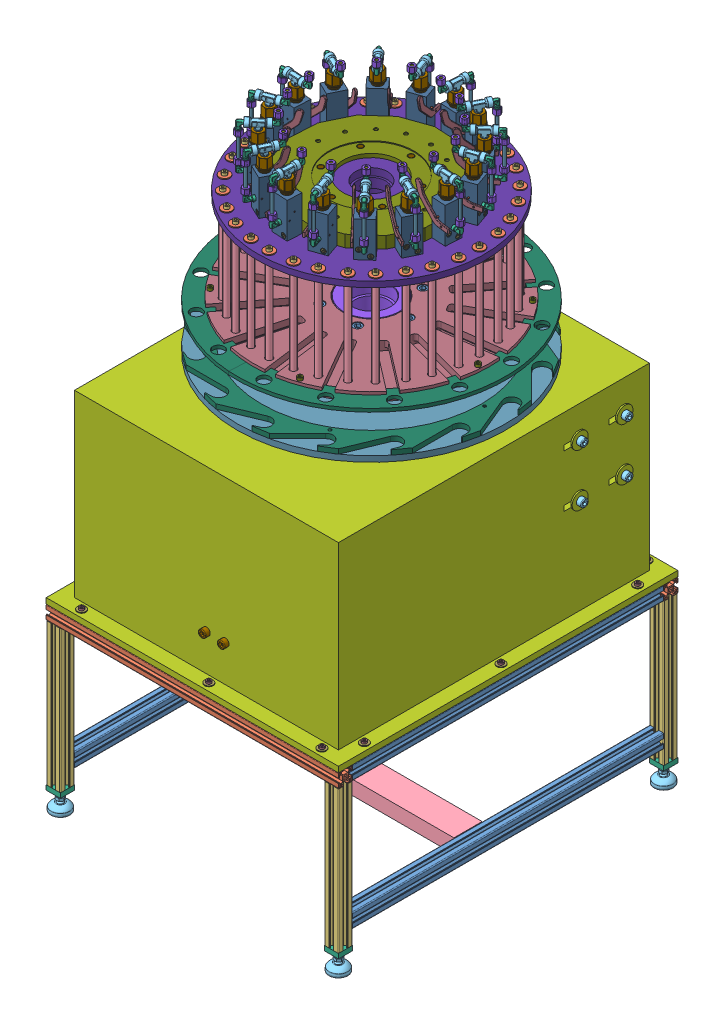
SolidWorks assembly Assieme_FINALE, configuration Default. Lengths in mm. (continued)
Components (placement in the parent): (continued)
- assieme parte rotante-1: assieme parte rotante [Default] at (-376.3498 623.9178 -790.5811) x (0 1 0) z (0 0 1) size (749.63 778.63 778.63) (continued)
  - AssiemeValvola-4: AssiemeValvola [Default] at (515.3257 -108.3081 301.6234) x (0 0.745128 0.666921) z (0 0.666921 -0.745128) size (90.26 138.63 38) (continued)
    - Raccordo a L-3: Raccordo a L [Default] at (-30 -88.2824 0) x (0 1 0) z (0 0 1) size (28.34 25.51 14.01)
      - 1809_06_10_01-1: 1809_06_10_01 [Default] at origin size (22.49 23 10)
      - 1809_06_10_02-1: 1809_06_10_02 [Default] at origin size (6.5 8.5 8.5)
      - 1809_06_10_03-1: 1809_06_10_03 [Default] at origin size (11.02 15.01 14.01)
    - Spina_3x38-1: Spina_3x38 [Default] at (0 -68.2824 -21) x (-1 0 0) z (0 0 1) size (3 3 38)
    - Spina_3x38-2: Spina_3x38 [Default] at (-10 -80.2824 -21) x (0.996193 0.087174 0) z (0 0 1) size (3 3 38)
    - M5 40mm-3: M5 40mm [ISO 4762 M5 x 40 - 40N] at (-14.6 -108.7824 9) size (45 8.5 8.5)
    - M5 40mm-2: M5 40mm [ISO 4762 M5 x 40 - 40N] at (-14.6 -96.7824 -9) size (45 8.5 8.5)
    - LevaValvola-1: LevaValvola [Default] at (-24.507 -86.571 -17) x (0.996193 0.087174 0) z (0 0 1) size (77.55 60.2 4)
    - Tubo-1: Tubo [Default] at (-30 -15.9665 0) x (1 0 0) z (0 -1 0) size (6 6 56.4)
  - AssiemeValvola-5: AssiemeValvola [Default] at (515.3257 -142.0531 358.7289) x (0 0.943628 0.331007) z (0 0.331007 -0.943628) size (90.26 138.63 38)
    - RaccordoT-1: RaccordoT [Default] at origin size (43 29.75 16.5)
    - Raccordo a L-1: Raccordo a L [Default] at (-30 0 0) x (0 -1 0) z (0 0 -1) size (28.34 25.51 14.01)
      - 1809_06_10_01-1: 1809_06_10_01 [Default] at origin size (22.49 23 10)
      - 1809_06_10_02-1: 1809_06_10_02 [Default] at origin size (6.5 8.5 8.5)
      - 1809_06_10_03-1: 1809_06_10_03 [Default] at origin size (11.02 15.01 14.01)
    - Raccordo a L-2: Raccordo a L [Default] at (30 0 0) x (0 1 0) z (0 0 -1) size (28.34 25.51 14.01)
      - 1809_06_10_01-1: 1809_06_10_01 [Default] at origin size (22.49 23 10)
      - 1809_06_10_02-1: 1809_06_10_02 [Default] at origin size (6.5 8.5 8.5)
      - 1809_06_10_03-1: 1809_06_10_03 [Default] at origin size (11.02 15.01 14.01)
    - TappoChiusura-1: TappoChiusura [Default] at (0 -32 0) x (0 -1 0) z (0 0 1) size (38.28 26.74 26.74)
    - CorpoValvola-1: CorpoValvola [Default] at (-15 -115.2824 0) size (30 75 34)
    - Raccordo a L-3: Raccordo a L [Default] at (-30 -88.2824 0) x (0 1 0) z (0 0 1) size (28.34 25.51 14.01)
      - 1809_06_10_01-1: 1809_06_10_01 [Default] at origin size (22.49 23 10)
      - 1809_06_10_02-1: 1809_06_10_02 [Default] at origin size (6.5 8.5 8.5)
      - 1809_06_10_03-1: 1809_06_10_03 [Default] at origin size (11.02 15.01 14.01)
    - Spina_3x38-1: Spina_3x38 [Default] at (0 -68.2824 -21) x (-1 0 0) z (0 0 1) size (3 3 38)
    - Spina_3x38-2: Spina_3x38 [Default] at (-10 -80.2824 -21) x (0.996193 0.087174 0) z (0 0 1) size (3 3 38)
    - M5 40mm-3: M5 40mm [ISO 4762 M5 x 40 - 40N] at (-14.6 -108.7824 9) size (45 8.5 8.5)
    - M5 40mm-2: M5 40mm [ISO 4762 M5 x 40 - 40N] at (-14.6 -96.7824 -9) size (45 8.5 8.5)
    - LevaValvola-1: LevaValvola [Default] at (-24.507 -86.571 -17) x (0.996193 0.087174 0) z (0 0 1) size (77.55 60.2 4)
    - Tubo-1: Tubo [Default] at (-30 -15.9665 0) x (1 0 0) z (0 -1 0) size (6 6 56.4)
  - AssiemeValvola-6: AssiemeValvola [Default] at (515.3257 -151.3762 424.4011) x (0 0.99847 -0.055301) z (0 -0.055301 -0.99847) size (90.26 138.63 38)
    - RaccordoT-1: RaccordoT [Default] at origin size (43 29.75 16.5)
    - Raccordo a L-1: Raccordo a L [Default] at (-30 0 0) x (0 -1 0) z (0 0 -1) size (28.34 25.51 14.01)
      - 1809_06_10_01-1: 1809_06_10_01 [Default] at origin size (22.49 23 10)
      - 1809_06_10_02-1: 1809_06_10_02 [Default] at origin size (6.5 8.5 8.5)
      - 1809_06_10_03-1: 1809_06_10_03 [Default] at origin size (11.02 15.01 14.01)
    - Raccordo a L-2: Raccordo a L [Default] at (30 0 0) x (0 1 0) z (0 0 -1) size (28.34 25.51 14.01)
      - 1809_06_10_01-1: 1809_06_10_01 [Default] at origin size (22.49 23 10)
      - 1809_06_10_02-1: 1809_06_10_02 [Default] at origin size (6.5 8.5 8.5)
      - 1809_06_10_03-1: 1809_06_10_03 [Default] at origin size (11.02 15.01 14.01)
    - TappoChiusura-1: TappoChiusura [Default] at (0 -32 0) x (0 -1 0) z (0 0 1) size (38.28 26.74 26.74)
    - CorpoValvola-1: CorpoValvola [Default] at (-15 -115.2824 0) size (30 75 34)
    - Raccordo a L-3: Raccordo a L [Default] at (-30 -88.2824 0) x (0 1 0) z (0 0 1) size (28.34 25.51 14.01)
      - 1809_06_10_01-1: 1809_06_10_01 [Default] at origin size (22.49 23 10)
      - 1809_06_10_02-1: 1809_06_10_02 [Default] at origin size (6.5 8.5 8.5)
      - 1809_06_10_03-1: 1809_06_10_03 [Default] at origin size (11.02 15.01 14.01)
    - Spina_3x38-1: Spina_3x38 [Default] at (0 -68.2824 -21) x (-1 0 0) z (0 0 1) size (3 3 38)
    - Spina_3x38-2: Spina_3x38 [Default] at (-10 -80.2824 -21) x (0.996193 0.087174 0) z (0 0 1) size (3 3 38)
    - M5 40mm-3: M5 40mm [ISO 4762 M5 x 40 - 40N] at (-14.6 -108.7824 9) size (45 8.5 8.5)
    - M5 40mm-2: M5 40mm [ISO 4762 M5 x 40 - 40N] at (-14.6 -96.7824 -9) size (45 8.5 8.5)
    - LevaValvola-1: LevaValvola [Default] at (-24.507 -86.571 -17) x (0.996193 0.087174 0) z (0 0 1) size (77.55 60.2 4)
    - Tubo-1: Tubo [Default] at (-30 -15.9665 0) x (1 0 0) z (0 -1 0) size (6 6 56.4)
  - AssiemeValvola-7: AssiemeValvola [Default] at (515.3257 -134.8578 488.6421) x (0 0.901303 -0.433189) z (0 -0.433189 -0.901303) size (90.26 138.63 38)
    - RaccordoT-1: RaccordoT [Default] at origin size (43 29.75 16.5)
    - Raccordo a L-1: Raccordo a L [Default] at (-30 0 0) x (0 -1 0) z (0 0 -1) size (28.34 25.51 14.01)
      - 1809_06_10_01-1: 1809_06_10_01 [Default] at origin size (22.49 23 10)
      - 1809_06_10_02-1: 1809_06_10_02 [Default] at origin size (6.5 8.5 8.5)
      - 1809_06_10_03-1: 1809_06_10_03 [Default] at origin size (11.02 15.01 14.01)
    - Raccordo a L-2: Raccordo a L [Default] at (30 0 0) x (0 1 0) z (0 0 -1) size (28.34 25.51 14.01)
      - 1809_06_10_01-1: 1809_06_10_01 [Default] at origin size (22.49 23 10)
      - 1809_06_10_02-1: 1809_06_10_02 [Default] at origin size (6.5 8.5 8.5)
      - 1809_06_10_03-1: 1809_06_10_03 [Default] at origin size (11.02 15.01 14.01)
    - TappoChiusura-1: TappoChiusura [Default] at (0 -32 0) x (0 -1 0) z (0 0 1) size (38.28 26.74 26.74)
    - CorpoValvola-1: CorpoValvola [Default] at (-15 -115.2824 0) size (30 75 34)
    - Raccordo a L-3: Raccordo a L [Default] at (-30 -88.2824 0) x (0 1 0) z (0 0 1) size (28.34 25.51 14.01)
      - 1809_06_10_01-1: 1809_06_10_01 [Default] at origin size (22.49 23 10)
      - 1809_06_10_02-1: 1809_06_10_02 [Default] at origin size (6.5 8.5 8.5)
      - 1809_06_10_03-1: 1809_06_10_03 [Default] at origin size (11.02 15.01 14.01)
    - Spina_3x38-1: Spina_3x38 [Default] at (0 -68.2824 -21) x (-1 0 0) z (0 0 1) size (3 3 38)
    - Spina_3x38-2: Spina_3x38 [Default] at (-10 -80.2824 -21) x (0.996193 0.087174 0) z (0 0 1) size (3 3 38)
    - M5 40mm-3: M5 40mm [ISO 4762 M5 x 40 - 40N] at (-14.6 -108.7824 9) size (45 8.5 8.5)
    - M5 40mm-2: M5 40mm [ISO 4762 M5 x 40 - 40N] at (-14.6 -96.7824 -9) size (45 8.5 8.5)
    - LevaValvola-1: LevaValvola [Default] at (-24.507 -86.571 -17) x (0.996193 0.087174 0) z (0 0 1) size (77.55 60.2 4)
    - Tubo-1: Tubo [Default] at (-30 -15.9665 0) x (1 0 0) z (0 -1 0) size (6 6 56.4)
  - AssiemeValvola-8: AssiemeValvola [Default] at (515.3257 -95.0129 541.6718) x (0 0.666921 -0.745128) z (0 -0.745128 -0.666921) size (90.26 138.63 38)
    - RaccordoT-1: RaccordoT [Default] at origin size (43 29.75 16.5)
    - Raccordo a L-1: Raccordo a L [Default] at (-30 0 0) x (0 -1 0) z (0 0 -1) size (28.34 25.51 14.01)
      - 1809_06_10_01-1: 1809_06_10_01 [Default] at origin size (22.49 23 10)
      - 1809_06_10_02-1: 1809_06_10_02 [Default] at origin size (6.5 8.5 8.5)
      - 1809_06_10_03-1: 1809_06_10_03 [Default] at origin size (11.02 15.01 14.01)
    - Raccordo a L-2: Raccordo a L [Default] at (30 0 0) x (0 1 0) z (0 0 -1) size (28.34 25.51 14.01)
      - 1809_06_10_01-1: 1809_06_10_01 [Default] at origin size (22.49 23 10)
      - 1809_06_10_02-1: 1809_06_10_02 [Default] at origin size (6.5 8.5 8.5)
      - 1809_06_10_03-1: 1809_06_10_03 [Default] at origin size (11.02 15.01 14.01)
    - TappoChiusura-1: TappoChiusura [Default] at (0 -32 0) x (0 -1 0) z (0 0 1) size (38.28 26.74 26.74)
    - CorpoValvola-1: CorpoValvola [Default] at (-15 -115.2824 0) size (30 75 34)
    - Raccordo a L-3: Raccordo a L [Default] at (-30 -88.2824 0) x (0 1 0) z (0 0 1) size (28.34 25.51 14.01)
      - 1809_06_10_01-1: 1809_06_10_01 [Default] at origin size (22.49 23 10)
      - 1809_06_10_02-1: 1809_06_10_02 [Default] at origin size (6.5 8.5 8.5)
      - 1809_06_10_03-1: 1809_06_10_03 [Default] at origin size (11.02 15.01 14.01)
    - Spina_3x38-1: Spina_3x38 [Default] at (0 -68.2824 -21) x (-1 0 0) z (0 0 1) size (3 3 38)
    - Spina_3x38-2: Spina_3x38 [Default] at (-10 -80.2824 -21) x (0.996193 0.087174 0) z (0 0 1) size (3 3 38)
    - M5 40mm-3: M5 40mm [ISO 4762 M5 x 40 - 40N] at (-14.6 -108.7824 9) size (45 8.5 8.5)
    - M5 40mm-2: M5 40mm [ISO 4762 M5 x 40 - 40N] at (-14.6 -96.7824 -9) size (45 8.5 8.5)
    - LevaValvola-1: LevaValvola [Default] at (-24.507 -86.571 -17) x (0.996193 0.087174 0) z (0 0 1) size (77.55 60.2 4)
    - Tubo-1: Tubo [Default] at (-30 -15.9665 0) x (1 0 0) z (0 -1 0) size (6 6 56.4)
  - AssiemeValvola-9: AssiemeValvola [Default] at (515.3257 -37.9074 575.4168) x (0 0.331007 -0.943628) z (0 -0.943628 -0.331007) size (90.26 138.63 38)
    - RaccordoT-1: RaccordoT [Default] at origin size (43 29.75 16.5)
    - Raccordo a L-1: Raccordo a L [Default] at (-30 0 0) x (0 -1 0) z (0 0 -1) size (28.34 25.51 14.01)
      - 1809_06_10_01-1: 1809_06_10_01 [Default] at origin size (22.49 23 10)
      - 1809_06_10_02-1: 1809_06_10_02 [Default] at origin size (6.5 8.5 8.5)
      - 1809_06_10_03-1: 1809_06_10_03 [Default] at origin size (11.02 15.01 14.01)
    - Raccordo a L-2: Raccordo a L [Default] at (30 0 0) x (0 1 0) z (0 0 -1) size (28.34 25.51 14.01)
      - 1809_06_10_01-1: 1809_06_10_01 [Default] at origin size (22.49 23 10)
      - 1809_06_10_02-1: 1809_06_10_02 [Default] at origin size (6.5 8.5 8.5)
      - 1809_06_10_03-1: 1809_06_10_03 [Default] at origin size (11.02 15.01 14.01)
    - TappoChiusura-1: TappoChiusura [Default] at (0 -32 0) x (0 -1 0) z (0 0 1) size (38.28 26.74 26.74)
    - CorpoValvola-1: CorpoValvola [Default] at (-15 -115.2824 0) size (30 75 34)
    - Raccordo a L-3: Raccordo a L [Default] at (-30 -88.2824 0) x (0 1 0) z (0 0 1) size (28.34 25.51 14.01)
      - 1809_06_10_01-1: 1809_06_10_01 [Default] at origin size (22.49 23 10)
      - 1809_06_10_02-1: 1809_06_10_02 [Default] at origin size (6.5 8.5 8.5)
      - 1809_06_10_03-1: 1809_06_10_03 [Default] at origin size (11.02 15.01 14.01)
    - Spina_3x38-1: Spina_3x38 [Default] at (0 -68.2824 -21) x (-1 0 0) z (0 0 1) size (3 3 38)
    - Spina_3x38-2: Spina_3x38 [Default] at (-10 -80.2824 -21) x (0.996193 0.087174 0) z (0 0 1) size (3 3 38)
    - M5 40mm-3: M5 40mm [ISO 4762 M5 x 40 - 40N] at (-14.6 -108.7824 9) size (45 8.5 8.5)
    - M5 40mm-2: M5 40mm [ISO 4762 M5 x 40 - 40N] at (-14.6 -96.7824 -9) size (45 8.5 8.5)
    - LevaValvola-1: LevaValvola [Default] at (-24.507 -86.571 -17) x (0.996193 0.087174 0) z (0 0 1) size (77.55 60.2 4)
    - Tubo-1: Tubo [Default] at (-30 -15.9665 0) x (1 0 0) z (0 -1 0) size (6 6 56.4)
  - AssiemeValvola-10: AssiemeValvola [Default] at (515.3257 27.7648 584.7399) x (0 -0.055301 -0.99847) z (0 -0.99847 0.055301) size (90.26 138.63 38)
    - RaccordoT-1: RaccordoT [Default] at origin size (43 29.75 16.5)
    - Raccordo a L-1: Raccordo a L [Default] at (-30 0 0) x (0 -1 0) z (0 0 -1) size (28.34 25.51 14.01)
      - 1809_06_10_01-1: 1809_06_10_01 [Default] at origin size (22.49 23 10)
      - 1809_06_10_02-1: 1809_06_10_02 [Default] at origin size (6.5 8.5 8.5)
      - 1809_06_10_03-1: 1809_06_10_03 [Default] at origin size (11.02 15.01 14.01)
    - Raccordo a L-2: Raccordo a L [Default] at (30 0 0) x (0 1 0) z (0 0 -1) size (28.34 25.51 14.01)
      - 1809_06_10_01-1: 1809_06_10_01 [Default] at origin size (22.49 23 10)
      - 1809_06_10_02-1: 1809_06_10_02 [Default] at origin size (6.5 8.5 8.5)
      - 1809_06_10_03-1: 1809_06_10_03 [Default] at origin size (11.02 15.01 14.01)
    - TappoChiusura-1: TappoChiusura [Default] at (0 -32 0) x (0 -1 0) z (0 0 1) size (38.28 26.74 26.74)
    - CorpoValvola-1: CorpoValvola [Default] at (-15 -115.2824 0) size (30 75 34)
    - Raccordo a L-3: Raccordo a L [Default] at (-30 -88.2824 0) x (0 1 0) z (0 0 1) size (28.34 25.51 14.01)
      - 1809_06_10_01-1: 1809_06_10_01 [Default] at origin size (22.49 23 10)
      - 1809_06_10_02-1: 1809_06_10_02 [Default] at origin size (6.5 8.5 8.5)
      - 1809_06_10_03-1: 1809_06_10_03 [Default] at origin size (11.02 15.01 14.01)
    - Spina_3x38-1: Spina_3x38 [Default] at (0 -68.2824 -21) x (-1 0 0) z (0 0 1) size (3 3 38)
    - Spina_3x38-2: Spina_3x38 [Default] at (-10 -80.2824 -21) x (0.996193 0.087174 0) z (0 0 1) size (3 3 38)
    - M5 40mm-3: M5 40mm [ISO 4762 M5 x 40 - 40N] at (-14.6 -108.7824 9) size (45 8.5 8.5)
    - M5 40mm-2: M5 40mm [ISO 4762 M5 x 40 - 40N] at (-14.6 -96.7824 -9) size (45 8.5 8.5)
    - LevaValvola-1: LevaValvola [Default] at (-24.507 -86.571 -17) x (0.996193 0.087174 0) z (0 0 1) size (77.55 60.2 4)
    - Tubo-1: Tubo [Default] at (-30 -15.9665 0) x (1 0 0) z (0 -1 0) size (6 6 56.4)
  - AssiemeValvola-11: AssiemeValvola [Default] at (515.3257 92.0058 568.2215) x (0 -0.433189 -0.901303) z (0 -0.901303 0.433189) size (90.26 138.63 38)
    - RaccordoT-1: RaccordoT [Default] at origin size (43 29.75 16.5)
    - Raccordo a L-1: Raccordo a L [Default] at (-30 0 0) x (0 -1 0) z (0 0 -1) size (28.34 25.51 14.01)
      - 1809_06_10_01-1: 1809_06_10_01 [Default] at origin size (22.49 23 10)
      - 1809_06_10_02-1: 1809_06_10_02 [Default] at origin size (6.5 8.5 8.5)
      - 1809_06_10_03-1: 1809_06_10_03 [Default] at origin size (11.02 15.01 14.01)
    - Raccordo a L-2: Raccordo a L [Default] at (30 0 0) x (0 1 0) z (0 0 -1) size (28.34 25.51 14.01)
      - 1809_06_10_01-1: 1809_06_10_01 [Default] at origin size (22.49 23 10)
      - 1809_06_10_02-1: 1809_06_10_02 [Default] at origin size (6.5 8.5 8.5)
      - 1809_06_10_03-1: 1809_06_10_03 [Default] at origin size (11.02 15.01 14.01)
    - TappoChiusura-1: TappoChiusura [Default] at (0 -32 0) x (0 -1 0) z (0 0 1) size (38.28 26.74 26.74)
    - CorpoValvola-1: CorpoValvola [Default] at (-15 -115.2824 0) size (30 75 34)
    - Raccordo a L-3: Raccordo a L [Default] at (-30 -88.2824 0) x (0 1 0) z (0 0 1) size (28.34 25.51 14.01)
      - 1809_06_10_01-1: 1809_06_10_01 [Default] at origin size (22.49 23 10)
      - 1809_06_10_02-1: 1809_06_10_02 [Default] at origin size (6.5 8.5 8.5)
      - 1809_06_10_03-1: 1809_06_10_03 [Default] at origin size (11.02 15.01 14.01)
    - Spina_3x38-1: Spina_3x38 [Default] at (0 -68.2824 -21) x (-1 0 0) z (0 0 1) size (3 3 38)
    - Spina_3x38-2: Spina_3x38 [Default] at (-10 -80.2824 -21) x (0.996193 0.087174 0) z (0 0 1) size (3 3 38)
    - M5 40mm-3: M5 40mm [ISO 4762 M5 x 40 - 40N] at (-14.6 -108.7824 9) size (45 8.5 8.5)
    - M5 40mm-2: M5 40mm [ISO 4762 M5 x 40 - 40N] at (-14.6 -96.7824 -9) size (45 8.5 8.5)
    - LevaValvola-1: LevaValvola [Default] at (-24.507 -86.571 -17) x (0.996193 0.087174 0) z (0 0 1) size (77.55 60.2 4)
    - Tubo-1: Tubo [Default] at (-30 -15.9665 0) x (1 0 0) z (0 -1 0) size (6 6 56.4)
  - AssiemeValvola-12: AssiemeValvola [Default] at (515.3257 145.0355 528.3766) x (0 -0.745128 -0.666921) z (0 -0.666921 0.745128) size (90.26 138.63 38)
    - RaccordoT-1: RaccordoT [Default] at origin size (43 29.75 16.5)
    - Raccordo a L-1: Raccordo a L [Default] at (-30 0 0) x (0 -1 0) z (0 0 -1) size (28.34 25.51 14.01)
      - 1809_06_10_01-1: 1809_06_10_01 [Default] at origin size (22.49 23 10)
      - 1809_06_10_02-1: 1809_06_10_02 [Default] at origin size (6.5 8.5 8.5)
      - 1809_06_10_03-1: 1809_06_10_03 [Default] at origin size (11.02 15.01 14.01)
    - Raccordo a L-2: Raccordo a L [Default] at (30 0 0) x (0 1 0) z (0 0 -1) size (28.34 25.51 14.01)
      - 1809_06_10_01-1: 1809_06_10_01 [Default] at origin size (22.49 23 10)
      - 1809_06_10_02-1: 1809_06_10_02 [Default] at origin size (6.5 8.5 8.5)
      - 1809_06_10_03-1: 1809_06_10_03 [Default] at origin size (11.02 15.01 14.01)
    - TappoChiusura-1: TappoChiusura [Default] at (0 -32 0) x (0 -1 0) z (0 0 1) size (38.28 26.74 26.74)
    - CorpoValvola-1: CorpoValvola [Default] at (-15 -115.2824 0) size (30 75 34)
    - Raccordo a L-3: Raccordo a L [Default] at (-30 -88.2824 0) x (0 1 0) z (0 0 1) size (28.34 25.51 14.01)
      - 1809_06_10_01-1: 1809_06_10_01 [Default] at origin size (22.49 23 10)
      - 1809_06_10_02-1: 1809_06_10_02 [Default] at origin size (6.5 8.5 8.5)
      - 1809_06_10_03-1: 1809_06_10_03 [Default] at origin size (11.02 15.01 14.01)
    - Spina_3x38-1: Spina_3x38 [Default] at (0 -68.2824 -21) x (-1 0 0) z (0 0 1) size (3 3 38)
    - Spina_3x38-2: Spina_3x38 [Default] at (-10 -80.2824 -21) x (0.996193 0.087174 0) z (0 0 1) size (3 3 38)
    - M5 40mm-3: M5 40mm [ISO 4762 M5 x 40 - 40N] at (-14.6 -108.7824 9) size (45 8.5 8.5)
    - M5 40mm-2: M5 40mm [ISO 4762 M5 x 40 - 40N] at (-14.6 -96.7824 -9) size (45 8.5 8.5)
    - LevaValvola-1: LevaValvola [Default] at (-24.507 -86.571 -17) x (0.996193 0.087174 0) z (0 0 1) size (77.55 60.2 4)
    - Tubo-1: Tubo [Default] at (-30 -15.9665 0) x (1 0 0) z (0 -1 0) size (6 6 56.4)
  - AssiemeValvola-13: AssiemeValvola [Default] at (515.3257 178.7805 471.2711) x (0 -0.943628 -0.331007) z (0 -0.331007 0.943628) size (90.26 138.63 38)
    - RaccordoT-1: RaccordoT [Default] at origin size (43 29.75 16.5)
    - Raccordo a L-1: Raccordo a L [Default] at (-30 0 0) x (0 -1 0) z (0 0 -1) size (28.34 25.51 14.01)
      - 1809_06_10_01-1: 1809_06_10_01 [Default] at origin size (22.49 23 10)
      - 1809_06_10_02-1: 1809_06_10_02 [Default] at origin size (6.5 8.5 8.5)
      - 1809_06_10_03-1: 1809_06_10_03 [Default] at origin size (11.02 15.01 14.01)
    - Raccordo a L-2: Raccordo a L [Default] at (30 0 0) x (0 1 0) z (0 0 -1) size (28.34 25.51 14.01)
      - 1809_06_10_01-1: 1809_06_10_01 [Default] at origin size (22.49 23 10)
      - 1809_06_10_02-1: 1809_06_10_02 [Default] at origin size (6.5 8.5 8.5)
      - 1809_06_10_03-1: 1809_06_10_03 [Default] at origin size (11.02 15.01 14.01)
    - TappoChiusura-1: TappoChiusura [Default] at (0 -32 0) x (0 -1 0) z (0 0 1) size (38.28 26.74 26.74)
    - CorpoValvola-1: CorpoValvola [Default] at (-15 -115.2824 0) size (30 75 34)
    - Raccordo a L-3: Raccordo a L [Default] at (-30 -88.2824 0) x (0 1 0) z (0 0 1) size (28.34 25.51 14.01)
      - 1809_06_10_01-1: 1809_06_10_01 [Default] at origin size (22.49 23 10)
      - 1809_06_10_02-1: 1809_06_10_02 [Default] at origin size (6.5 8.5 8.5)
      - 1809_06_10_03-1: 1809_06_10_03 [Default] at origin size (11.02 15.01 14.01)
    - Spina_3x38-1: Spina_3x38 [Default] at (0 -68.2824 -21) x (-1 0 0) z (0 0 1) size (3 3 38)
    - Spina_3x38-2: Spina_3x38 [Default] at (-10 -80.2824 -21) x (0.996193 0.087174 0) z (0 0 1) size (3 3 38)
    - M5 40mm-3: M5 40mm [ISO 4762 M5 x 40 - 40N] at (-14.6 -108.7824 9) size (45 8.5 8.5)
    - M5 40mm-2: M5 40mm [ISO 4762 M5 x 40 - 40N] at (-14.6 -96.7824 -9) size (45 8.5 8.5)
    - LevaValvola-1: LevaValvola [Default] at (-24.507 -86.571 -17) x (0.996193 0.087174 0) z (0 0 1) size (77.55 60.2 4)
    - Tubo-1: Tubo [Default] at (-30 -15.9665 0) x (1 0 0) z (0 -1 0) size (6 6 56.4)
  - AssiemeValvola-14: AssiemeValvola [Default] at (515.3257 188.1036 405.5989) x (0 -0.99847 0.055301) z (0 0.055301 0.99847) size (90.26 138.63 38)
    - RaccordoT-1: RaccordoT [Default] at origin size (43 29.75 16.5)
    - Raccordo a L-1: Raccordo a L [Default] at (-30 0 0) x (0 -1 0) z (0 0 -1) size (28.34 25.51 14.01)
      - 1809_06_10_01-1: 1809_06_10_01 [Default] at origin size (22.49 23 10)
      - 1809_06_10_02-1: 1809_06_10_02 [Default] at origin size (6.5 8.5 8.5)
      - 1809_06_10_03-1: 1809_06_10_03 [Default] at origin size (11.02 15.01 14.01)
    - Raccordo a L-2: Raccordo a L [Default] at (30 0 0) x (0 1 0) z (0 0 -1) size (28.34 25.51 14.01)
      - 1809_06_10_01-1: 1809_06_10_01 [Default] at origin size (22.49 23 10)
      - 1809_06_10_02-1: 1809_06_10_02 [Default] at origin size (6.5 8.5 8.5)
      - 1809_06_10_03-1: 1809_06_10_03 [Default] at origin size (11.02 15.01 14.01)
    - TappoChiusura-1: TappoChiusura [Default] at (0 -32 0) x (0 -1 0) z (0 0 1) size (38.28 26.74 26.74)
    - CorpoValvola-1: CorpoValvola [Default] at (-15 -115.2824 0) size (30 75 34)
    - Raccordo a L-3: Raccordo a L [Default] at (-30 -88.2824 0) x (0 1 0) z (0 0 1) size (28.34 25.51 14.01)
      - 1809_06_10_01-1: 1809_06_10_01 [Default] at origin size (22.49 23 10)
      - 1809_06_10_02-1: 1809_06_10_02 [Default] at origin size (6.5 8.5 8.5)
      - 1809_06_10_03-1: 1809_06_10_03 [Default] at origin size (11.02 15.01 14.01)
    - Spina_3x38-1: Spina_3x38 [Default] at (0 -68.2824 -21) x (-1 0 0) z (0 0 1) size (3 3 38)
    - Spina_3x38-2: Spina_3x38 [Default] at (-10 -80.2824 -21) x (0.996193 0.087174 0) z (0 0 1) size (3 3 38)
    - M5 40mm-3: M5 40mm [ISO 4762 M5 x 40 - 40N] at (-14.6 -108.7824 9) size (45 8.5 8.5)
    - M5 40mm-2: M5 40mm [ISO 4762 M5 x 40 - 40N] at (-14.6 -96.7824 -9) size (45 8.5 8.5)
    - LevaValvola-1: LevaValvola [Default] at (-24.507 -86.571 -17) x (0.996193 0.087174 0) z (0 0 1) size (77.55 60.2 4)
    - Tubo-1: Tubo [Default] at (-30 -15.9665 0) x (1 0 0) z (0 -1 0) size (6 6 56.4)
  - AssiemeValvola-15: AssiemeValvola [Default] at (515.3257 171.5852 341.3579) x (0 -0.901303 0.433189) z (0 0.433189 0.901303) size (90.26 138.63 38)
    - RaccordoT-1: RaccordoT [Default] at origin size (43 29.75 16.5)
    - Raccordo a L-1: Raccordo a L [Default] at (-30 0 0) x (0 -1 0) z (0 0 -1) size (28.34 25.51 14.01)
      - 1809_06_10_01-1: 1809_06_10_01 [Default] at origin size (22.49 23 10)
      - 1809_06_10_02-1: 1809_06_10_02 [Default] at origin size (6.5 8.5 8.5)
      - 1809_06_10_03-1: 1809_06_10_03 [Default] at origin size (11.02 15.01 14.01)
    - Raccordo a L-2: Raccordo a L [Default] at (30 0 0) x (0 1 0) z (0 0 -1) size (28.34 25.51 14.01)
      - 1809_06_10_01-1: 1809_06_10_01 [Default] at origin size (22.49 23 10)
      - 1809_06_10_02-1: 1809_06_10_02 [Default] at origin size (6.5 8.5 8.5)
      - 1809_06_10_03-1: 1809_06_10_03 [Default] at origin size (11.02 15.01 14.01)
    - TappoChiusura-1: TappoChiusura [Default] at (0 -32 0) x (0 -1 0) z (0 0 1) size (38.28 26.74 26.74)
    - CorpoValvola-1: CorpoValvola [Default] at (-15 -115.2824 0) size (30 75 34)
    - Raccordo a L-3: Raccordo a L [Default] at (-30 -88.2824 0) x (0 1 0) z (0 0 1) size (28.34 25.51 14.01)
      - 1809_06_10_01-1: 1809_06_10_01 [Default] at origin size (22.49 23 10)
      - 1809_06_10_02-1: 1809_06_10_02 [Default] at origin size (6.5 8.5 8.5)
      - 1809_06_10_03-1: 1809_06_10_03 [Default] at origin size (11.02 15.01 14.01)
    - Spina_3x38-1: Spina_3x38 [Default] at (0 -68.2824 -21) x (-1 0 0) z (0 0 1) size (3 3 38)
    - Spina_3x38-2: Spina_3x38 [Default] at (-10 -80.2824 -21) x (0.996193 0.087174 0) z (0 0 1) size (3 3 38)
    - M5 40mm-3: M5 40mm [ISO 4762 M5 x 40 - 40N] at (-14.6 -108.7824 9) size (45 8.5 8.5)
    - M5 40mm-2: M5 40mm [ISO 4762 M5 x 40 - 40N] at (-14.6 -96.7824 -9) size (45 8.5 8.5)
    - LevaValvola-1: LevaValvola [Default] at (-24.507 -86.571 -17) x (0.996193 0.087174 0) z (0 0 1) size (77.55 60.2 4)
    - Tubo-1: Tubo [Default] at (-30 -15.9665 0) x (1 0 0) z (0 -1 0) size (6 6 56.4)
  - AssiemeValvola-16: AssiemeValvola [Default] at (515.3257 131.7403 288.3282) x (0 -0.666921 0.745128) z (0 0.745128 0.666921) size (90.26 138.63 38)
    - RaccordoT-1: RaccordoT [Default] at origin size (43 29.75 16.5)
    - Raccordo a L-1: Raccordo a L [Default] at (-30 0 0) x (0 -1 0) z (0 0 -1) size (28.34 25.51 14.01)
      - 1809_06_10_01-1: 1809_06_10_01 [Default] at origin size (22.49 23 10)
      - 1809_06_10_02-1: 1809_06_10_02 [Default] at origin size (6.5 8.5 8.5)
      - 1809_06_10_03-1: 1809_06_10_03 [Default] at origin size (11.02 15.01 14.01)
    - Raccordo a L-2: Raccordo a L [Default] at (30 0 0) x (0 1 0) z (0 0 -1) size (28.34 25.51 14.01)
      - 1809_06_10_01-1: 1809_06_10_01 [Default] at origin size (22.49 23 10)
      - 1809_06_10_02-1: 1809_06_10_02 [Default] at origin size (6.5 8.5 8.5)
      - 1809_06_10_03-1: 1809_06_10_03 [Default] at origin size (11.02 15.01 14.01)
    - TappoChiusura-1: TappoChiusura [Default] at (0 -32 0) x (0 -1 0) z (0 0 1) size (38.28 26.74 26.74)
    - CorpoValvola-1: CorpoValvola [Default] at (-15 -115.2824 0) size (30 75 34)
    - Raccordo a L-3: Raccordo a L [Default] at (-30 -88.2824 0) x (0 1 0) z (0 0 1) size (28.34 25.51 14.01)
      - 1809_06_10_01-1: 1809_06_10_01 [Default] at origin size (22.49 23 10)
      - 1809_06_10_02-1: 1809_06_10_02 [Default] at origin size (6.5 8.5 8.5)
      - 1809_06_10_03-1: 1809_06_10_03 [Default] at origin size (11.02 15.01 14.01)
    - Spina_3x38-1: Spina_3x38 [Default] at (0 -68.2824 -21) x (-1 0 0) z (0 0 1) size (3 3 38)
    - Spina_3x38-2: Spina_3x38 [Default] at (-10 -80.2824 -21) x (0.996193 0.087174 0) z (0 0 1) size (3 3 38)
    - M5 40mm-3: M5 40mm [ISO 4762 M5 x 40 - 40N] at (-14.6 -108.7824 9) size (45 8.5 8.5)
    - M5 40mm-2: M5 40mm [ISO 4762 M5 x 40 - 40N] at (-14.6 -96.7824 -9) size (45 8.5 8.5)
    - LevaValvola-1: LevaValvola [Default] at (-24.507 -86.571 -17) x (0.996193 0.087174 0) z (0 0 1) size (77.55 60.2 4)
    - Tubo-1: Tubo [Default] at (-30 -15.9665 0) x (1 0 0) z (0 -1 0) size (6 6 56.4)
  - Disco alimentazione guarnizione fi24.4-1: Disco alimentazione guarnizione fi24.4 [Default] at (198.0433 18.3637 415) x (0 0.065403 0.997859) z (-1 0 0) size (570 285 7.35)
  - Disco alimentazione guarnizione fi24.4-2: Disco alimentazione guarnizione fi24.4 [Default] at (198.0433 18.3637 415) x (0 -0.065403 -0.997859) z (-1 0 0) size (570 285 7.35)
  - m6 12mm-1: m6 12mm [ISO 4762 M6 x 12 - 12N] at (210.0433 200.6849 574.8914) x (-1 0 0) z (0 0.793353 -0.608761) size (18 10 10)
  - m6 12mm-7: m6 12mm [ISO 4762 M6 x 12 - 12N] at (210.0433 260.3445 399.1397) x (-1 0 0) z (0 0.793353 -0.608761) size (18 10 10)
  - m6 12mm-8: m6 12mm [ISO 4762 M6 x 12 - 12N] at (210.0433 96.3128 185.3694) x (-1 0 0) z (0 0.793353 -0.608761) size (18 10 10)
  - m6 12mm-9: m6 12mm [ISO 4762 M6 x 12 - 12N] at (210.0433 -59.5854 644.6306) x (-1 0 0) z (0 -0.793353 -0.608761) size (18 10 10)
  - m6 12mm-10: m6 12mm [ISO 4762 M6 x 12 - 12N] at (210.0433 -223.6171 430.8603) x (-1 0 0) z (0 -0.793353 -0.608761) size (18 10 10)
  - m6 12mm-11: m6 12mm [ISO 4762 M6 x 12 - 12N] at (210.0433 -163.9575 255.1086) x (-1 0 0) z (0 0.793353 -0.608761) size (18 10 10)
Mates (geometry in assembly coordinates):
- Parallelo2: parallel aligned: plane of SupportoBase_Totale-2 through (4.0127 -14.4529 -3.9361) normal (0 1 0)
- Perpendicolare1: perpendicular: plane of SupportoBase_Totale-2 through (4.0127 -14.4529 -3.9361) normal (0 1 0)
- Parallelo4: parallel aligned: plane of SupportoBase_Totale-2 through (4.0127 -14.4529 -3.9361) normal (0 0 1)
- Coincidente5: coincident anti-aligned: plane of SupportoBase_Totale-2/assieme_base-1/Supporto di Base per macchina-1 through (-154.7135 275.9611 -15.5811) normal (-1 0 0); plane of motoriduttore-1 through (-154.7135 275.9611 -1179.5811) normal (1 0 0)
- Coincidente6: coincident aligned: plane of SupportoBase_Totale-2/assieme_base-1/Supporto di Base per macchina-1 through (-154.7135 467.9611 -697.5811) normal (0 0 -1); plane of motoriduttore-1 through (-154.7135 463.6811 -697.5811) normal (0 0 -1)
- Tangente1: tangent anti-aligned: plane of SupportoBase_Totale-2/assieme_base-1/Supporto di Base per macchina-1 through (-93.2286 597.9611 -659.5811) normal (0 1 0); cylinder of motoriduttore-1 through (-154.7135 603.4611 -650.5811) axis (-1 0 0) radius 5.5
- Concentrico1: concentric anti-aligned: cylinder of motoriduttore-1 through (-267.2135 442.7547 -597.5811) axis (0 1 0) radius 15; cylinder of Assieme_Riduttore-1/AlberoRiduttore-1 through (-267.2135 379.4375 -597.5811) axis (0 -1 0) radius 12.5
- Coincidente9: coincident anti-aligned: plane of motoriduttore-1 through (-164.7135 602.1811 -1179.5811) normal (0 1 0); plane of Assieme_Riduttore-1/Rondella di fermo-2 through (-267.2135 602.1811 -597.5811) normal (0 -1 0)
- Coincidente12: coincident anti-aligned: plane of socket head cap screw_iso-1 through (-131.7135 606.5159 -562.9749) normal (-1 0 0); plane of plain washer xlarge grade c_iso-1 through (-131.7135 596.9697 -539.8693) normal (1 0 0)
- Concentrico4: concentric aligned: cylinder of socket head cap screw_iso-1 through (-89.9635 603.4611 -555.5811) axis (1 0 0) radius 5; cylinder of plain washer xlarge grade c_iso-1 through (-99.7885 603.4611 -555.5811) axis (1 0 0) radius 5.5
- Coincidente13: coincident anti-aligned: plane of socket head cap screw_iso-2 through (-131.7135 484.4611 -555.5811) normal (-1 0 0); plane of plain washer xlarge grade c_iso-2 through (-131.7135 475.4611 -555.5811) normal (1 0 0)
- Concentrico5: concentric aligned: cylinder of socket head cap screw_iso-2 through (-89.9635 492.4611 -555.5811) axis (1 0 0) radius 5; cylinder of plain washer xlarge grade c_iso-2 through (-99.7885 492.4611 -555.5811) axis (1 0 0) radius 5.5
- Coincidente14: coincident anti-aligned: plane of socket head cap screw_iso-3 through (-131.7135 595.4611 -650.5811) normal (-1 0 0); plane of plain washer xlarge grade c_iso-4 through (-131.7135 586.4611 -650.5811) normal (1 0 0)
- Concentrico6: concentric aligned: cylinder of socket head cap screw_iso-3 through (-89.9635 603.4611 -650.5811) axis (1 0 0) radius 5; cylinder of plain washer xlarge grade c_iso-4 through (-99.7885 603.4611 -650.5811) axis (1 0 0) radius 5.5
- Coincidente15: coincident anti-aligned: plane of socket head cap screw_iso-4 through (-131.7135 484.4611 -650.5811) normal (-1 0 0); plane of plain washer xlarge grade c_iso-3 through (-131.7135 475.4611 -650.5811) normal (1 0 0)
- Concentrico7: concentric aligned: cylinder of socket head cap screw_iso-4 through (-89.9635 492.4611 -650.5811) axis (1 0 0) radius 5; cylinder of plain washer xlarge grade c_iso-3 through (-99.7885 492.4611 -650.5811) axis (1 0 0) radius 5.5
- Concentrico8: concentric anti-aligned: cylinder of motoriduttore-1 through (-154.7135 603.4611 -650.5811) axis (-1 0 0) radius 5.5; cylinder of socket head cap screw_iso-3 through (-89.9635 603.4611 -650.5811) axis (1 0 0) radius 5
- Coincidente16: coincident anti-aligned: plane of SupportoBase_Totale-2/assieme_base-1/Supporto di Base per macchina-1 through (-134.7135 287.9611 -15.5811) normal (1 0 0); plane of plain washer xlarge grade c_iso-4 through (-134.7135 597.9611 -650.5811) normal (-1 0 0)
- Concentrico9: concentric anti-aligned: cylinder of motoriduttore-1 through (-154.7135 603.4611 -555.5811) axis (-1 0 0) radius 5.5; cylinder of socket head cap screw_iso-1 through (-89.9635 603.4611 -555.5811) axis (1 0 0) radius 5
- Coincidente17: coincident anti-aligned: plane of SupportoBase_Totale-2/assieme_base-1/Supporto di Base per macchina-1 through (-134.7135 287.9611 -15.5811) normal (1 0 0); plane of plain washer xlarge grade c_iso-1 through (-134.7135 601.3609 -550.4979) normal (-1 0 0)
- Coincidente18: coincident anti-aligned: plane of SupportoBase_Totale-2/assieme_base-1/Supporto di Base per macchina-1 through (-134.7135 287.9611 -15.5811) normal (1 0 0); plane of plain washer xlarge grade c_iso-3 through (-134.7135 486.9611 -650.5811) normal (-1 0 0)
- Concentrico10: concentric aligned: circle of motoriduttore-1; cylinder of socket head cap screw_iso-4 through (-89.9635 492.4611 -650.5811) axis (1 0 0) radius 5
- Coincidente19: coincident anti-aligned: plane of SupportoBase_Totale-2/assieme_base-1/Supporto di Base per macchina-1 through (-134.7135 287.9611 -15.5811) normal (1 0 0); plane of plain washer xlarge grade c_iso-2 through (-134.7135 486.9611 -555.5811) normal (-1 0 0)
- Concentrico11: concentric aligned: circle of motoriduttore-1; cylinder of socket head cap screw_iso-2 through (-89.9635 492.4611 -555.5811) axis (1 0 0) radius 5
- Concentrico12: concentric anti-aligned: cylinder of socket head cap screw_iso-4 through (-89.9635 492.4611 -650.5811) axis (1 0 0) radius 5; cylinder of hex nut style 2 gradeab_iso-3 through (-164.7135 492.4611 -650.5811) axis (-1 0 0) radius 4.25
- Coincidente20: coincident anti-aligned: plane of motoriduttore-1 through (-164.7135 275.9611 -1179.5811) normal (-1 0 0); plane of hex nut style 2 gradeab_iso-3 through (-164.7135 501.6987 -650.5811) normal (1 0 0)
- Concentrico13: concentric anti-aligned: cylinder of socket head cap screw_iso-3 through (-89.9635 603.4611 -650.5811) axis (1 0 0) radius 5; cylinder of hex nut style 2 gradeab_iso-1 through (-164.7135 603.4611 -650.5811) axis (-1 0 0) radius 4.25
- Coincidente21: coincident aligned: plane of motoriduttore-1 through (-164.7135 275.9611 -1179.5811) normal (-1 0 0); circle of hex nut style 2 gradeab_iso-1
- Concentrico14: concentric anti-aligned: cylinder of socket head cap screw_iso-1 through (-89.9635 603.4611 -555.5811) axis (1 0 0) radius 5; cylinder of hex nut style 2 gradeab_iso-2 through (-164.7135 603.4611 -555.5811) axis (-1 0 0) radius 4.25
- Coincidente22: coincident anti-aligned: plane of motoriduttore-1 through (-164.7135 275.9611 -1179.5811) normal (-1 0 0); plane of hex nut style 2 gradeab_iso-2 through (-164.7135 612.6987 -555.5811) normal (1 0 0)
- Concentrico15: concentric anti-aligned: cylinder of socket head cap screw_iso-2 through (-89.9635 492.4611 -555.5811) axis (1 0 0) radius 5; cylinder of hex nut style 2 gradeab_iso-4 through (-164.7135 492.4611 -555.5811) axis (-1 0 0) radius 4.25
- Coincidente23: coincident anti-aligned: plane of motoriduttore-1 through (-164.7135 275.9611 -1179.5811) normal (-1 0 0); plane of hex nut style 2 gradeab_iso-4 through (-164.7135 501.6987 -555.5811) normal (1 0 0)
- Concentrico161: concentric aligned: cylinder of SupportoBase_Totale-2/assieme_base-1/canotto di supporto-1 through (-394.7135 587.1745 -375.5811) axis (0 1 0) radius 119; cylinder of assieme parte fissa-1/dado M20-3 through (-394.7135 692.9236 -375.5811) axis (0 1 0) radius 10
- Coincidente241: coincident anti-aligned: plane of SupportoBase_Totale-2/assieme_base-1/canotto di supporto-1 through (-394.7135 698.9611 -375.5811) normal (0 1 0); plane of assieme parte fissa-1/dado M20-3 through (-409.2137 698.9611 -385.0544) normal (0 -1 0)
- Concentrico17: concentric aligned: cylinder of SupportoBase_Totale-2/assieme_base-1/canotto di supporto-1 through (-394.7135 587.1745 -375.5811) axis (0 1 0) radius 67.5; cylinder of assieme parte rotante-1/albero rotazione piatti-1 through (-394.7135 684.3308 -375.5811) axis (0 1 0) radius 49.75
- Coincidente25: coincident anti-aligned: plane of SupportoBase_Totale-2/assieme_base-1/canotto di supporto-1 through (-394.7135 673.9611 -375.5811) normal (0 1 0); plane of assieme parte rotante-1/SKF - 6020 - 20,DE,NC,20_68-2 through (-333.8574 673.9611 -346.3787) normal (0 -1 0)
